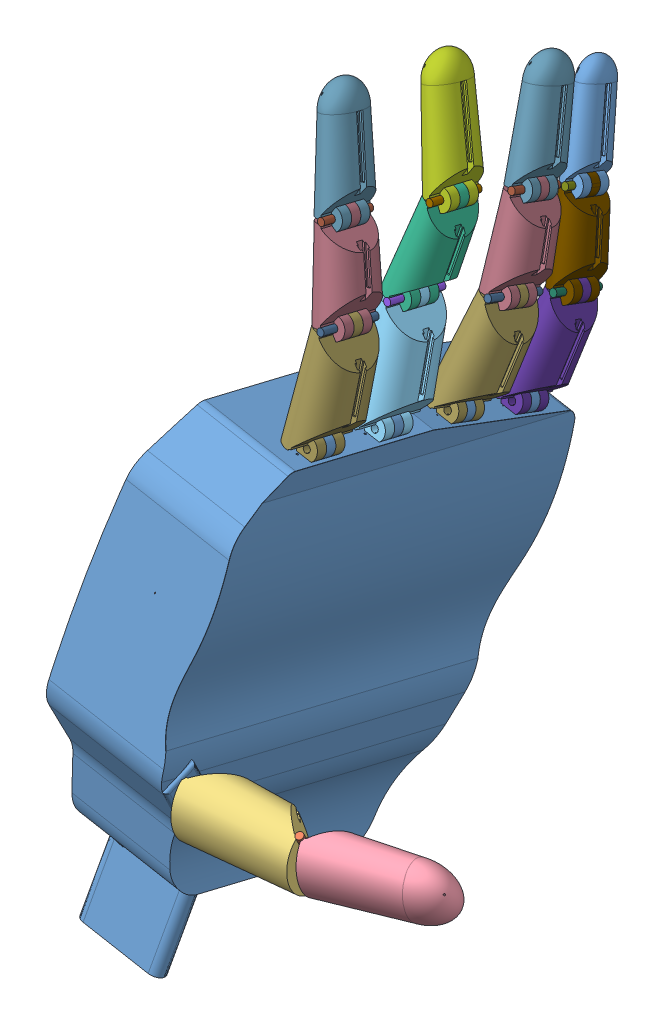
SolidWorks assembly hand_ass_son, configuration Default. Lengths in mm.
Overall size (126.68 238.36 164.71).
29 component instances, 20 part files, 48 mates.
Components (placement in the parent):
- mainbody_v2-4: mainbody_v2 [Default] at (1393.0939 256.2845 230.0733) x (-0.03967 -0.262646 -0.964076) z (0.98509 -0.171926 0.006304) size (116.82 140 48.77)
- Mate1t-4: Mate1t [Default] at (1443.7902 225.3063 267.9284) x (0.146425 0.857082 0.493933) z (0.670742 0.280983 -0.686407) size (23 2 2)
- Part1t-3: Part1t [Default] at (1431.2867 235.9478 276.4521) x (0.146425 0.857082 0.493933) z (-0.086451 0.508491 -0.856716) size (25.41 37 18.49)
- Part2t-3: Part2t [Default] at (1462.1105 235.1801 268.6506) x (0.146425 0.857082 0.493933) z (-0.264208 0.51506 -0.815419) size (22.13 38.57 15.06)
- Part1m-2: Part1m [Default] at (1414.4402 322.5973 216.192) x (-0.03967 -0.262646 -0.964076) z (0.999177 -0.002227 -0.040508) size (21.28 37 15.36)
- Part2m-2: Part2m [Default] at (1416.9612 349.6562 208.7166) x (-0.03967 -0.262646 -0.964076) z (0.980971 -0.193758 0.012421) size (18.99 32 13.25)
- Part3m-2: Part3m [Default] at (1414.6092 375.7736 201.6979) x (-0.03967 -0.262646 -0.964076) z (0.948609 0.293255 -0.118926) size (16.1 35.5 11.04)
- Mate1-2: Mate1 [Default] at (1415.2589 339.0559 221.0098) x (-0.03967 -0.262646 -0.964076) z (0.870094 0.465305 -0.162567) size (18 2 2)
- Mate2-2: Mate2 [Default] at (1420.1608 363.3694 213.1471) x (-0.03967 -0.262646 -0.964076) z (0.88018 0.447523 -0.158138) size (16 2 2)
- Mate1i-7: Mate1i [Default] at (1419.1567 328.7029 194.6213) x (-0.061096 -0.383846 -0.921374) z (0.853883 0.457912 -0.247388) size (18 2 2)
- Mate2i-7: Mate2i [Default] at (1415.3779 344.2512 169.9444) x (0.061096 0.383846 0.921374) z (-0.994886 0.097798 0.025228) size (16 2 2)
- Part1i-6: Part1i [Default] at (1415.7923 312.9467 191.6404) x (-0.061096 -0.383846 -0.921374) z (0.98509 -0.171926 0.006304) size (21.16 35 15.37)
- Part2-6: Part2 [Default] at (1416.6054 336.7334 181.6776) x (-0.061096 -0.383846 -0.921374) z (0.991581 0.082247 -0.100016) size (18.98 30 13.22)
- Part3i-6: Part3i [Default] at (1412.8163 360.7728 171.9137) x (-0.061096 -0.383846 -0.921374) z (0.980311 0.150581 -0.127736) size (16.1 33.51 11.04)
- Mate1p-2: Mate1p [Default] at (1417.5601 318.7755 173.3582) x (-0.061096 -0.383846 -0.921374) z (0.991721 -0.127797 -0.01252) size (16 2 2)
- Mate2p-2: Mate2p [Default] at (1411.96 339.126 164.166) x (-0.061096 -0.383846 -0.921374) z (0.997555 0.007899 -0.069439) size (14 2 2)
- Part1p-2: Part1p [Default] at (1414.4302 303.698 171.1644) x (-0.061096 -0.383846 -0.921374) z (0.98509 -0.171926 0.006304) size (18.99 34 13.27)
- Part2p-2: Part2p [Default] at (1413.7865 326.3018 161.7901) x (-0.061096 -0.383846 -0.921374) z (0.968644 0.199919 -0.147517) size (16.86 29 11.21)
- Part3p-2: Part3p [Default] at (1408.3506 348.6966 152.8208) x (-0.061096 -0.383846 -0.921374) z (0.974142 0.178236 -0.138849) size (14.11 31.5 9.04)
- Mate1i-8: Mate1i [Default] at (1416.3045 338.1976 225.4891) x (0.03967 0.262646 0.964076) z (-0.987081 -0.139593 0.078646) size (18 2 2)
- Mate2i-8: Mate2i [Default] at (1409.7839 360.8016 220.6372) x (0.03967 0.262646 0.964076) z (-0.919513 -0.368003 0.138092) size (16 2 2)
- Part1i-7: Part1i [Default] at (1415.7465 327.3903 237.7916) x (-0.03967 -0.262646 -0.964076) z (0.998985 -0.031014 -0.032657) size (21.16 35 15.37)
- Part3i-7: Part3i [Default] at (1405.8994 376.6502 224.7772) x (-0.03967 -0.262646 -0.964076) z (0.963202 0.246636 -0.106826) size (16.1 33.51 11.04)
- Part2-7: Part2 [Default] at (1412.6818 352.0877 231.19) x (-0.03967 -0.262646 -0.964076) z (0.961097 0.253914 -0.108722) size (18.98 30 13.22)
- SERVO 2-2: SERVO 2 [Default] at (1378.4658 252.7443 237.0888) x (0.374746 0.816954 0.438351) z (0.900147 -0.433837 0.039007) size (32 28.96 12.1)
- SERVO 2-3: SERVO 2 [Default] at (1410.6392 255.7893 252.4191) x (0.348093 0.174989 0.920983) z (-0.929377 0.193147 0.314567) size (32 28.96 12.1)
- SERVO 2-4: SERVO 2 [Default] at (1411.5824 241.8867 212.5876) x (0.093781 0.315033 0.944436) z (-0.990432 0.125987 0.056324) size (32 28.96 12.1)
- SERVO 2-6: SERVO 2 [Default] at (1414.0198 249.6937 180.1774) x (0.274408 0.279911 0.919973) z (-0.954781 0.193152 0.226022) size (32 28.96 12.1)
- SERVO 2-7: SERVO 2 [Default] at (1409.5967 265.7988 229.5325) x (0.0903 0.334214 0.938161) z (-0.97905 0.202412 0.022128) size (32 28.96 12.1)
Mates (geometry in assembly coordinates):
- Concentric1: concentric anti-aligned: cylinder of mainbody_v2-4 through (1415.9837 312.2001 240.3647) axis (0.03967 0.262646 0.964076) radius 1; cylinder of Part1i-7 through (1416.4652 315.3881 252.0667) axis (-0.03967 -0.262646 -0.964076) radius 1
- Coincident1: coincident anti-aligned: plane of mainbody_v2-4 through (1415.9837 312.2001 240.3647) normal (-0.03967 -0.262646 -0.964076); plane of Part1i-7 through (1415.9837 312.2001 240.3647) normal (0.03967 0.262646 0.964076)
- Concentric4: concentric aligned: cylinder of Part1i-7 through (1417.0836 343.3556 244.4221) axis (-0.03967 -0.262646 -0.964076) radius 1; cylinder of Part2-7 through (1417.0387 343.0583 243.331) axis (-0.03967 -0.262646 -0.964076) radius 1
- Coincident4: coincident anti-aligned: plane of Part1i-7 through (1416.6021 340.1676 232.72) normal (-0.03967 -0.262646 -0.964076); plane of Part2-7 through (1416.6021 340.1676 232.72) normal (0.03967 0.262646 0.964076)
- Concentric5: concentric aligned: cylinder of Mate1i-8 through (1417.0186 342.9252 242.8424) axis (-0.03967 -0.262646 -0.964076) radius 1; cylinder of Part2-7 through (1417.0387 343.0583 243.331) axis (-0.03967 -0.262646 -0.964076) radius 1
- Coincident5: coincident anti-aligned: plane of Mate1i-8 through (1416.6616 340.5614 234.1658) normal (0.03967 0.262646 0.964076); plane of Part1i-7 through (1415.7465 327.3903 237.7916) normal (-0.03967 -0.262646 -0.964076)
- Concentric6: concentric anti-aligned: cylinder of Part3i-7 through (1409.8037 360.9329 221.1191) axis (0.03967 0.262646 0.964076) radius 1; cylinder of Part2-7 through (1410.4784 365.3995 237.5145) axis (-0.03967 -0.262646 -0.964076) radius 1
- Coincident6: coincident anti-aligned: plane of Part3i-7 through (1410.0417 362.5088 226.9035) normal (0.03967 0.262646 0.964076); plane of Part2-7 through (1410.0417 362.5088 226.9035) normal (-0.03967 -0.262646 -0.964076)
- Concentric8: concentric anti-aligned: cylinder of Mate2i-8 through (1410.4186 365.004 236.0624) axis (-0.03967 -0.262646 -0.964076) radius 1; cylinder of Part3i-7 through (1409.8037 360.9329 221.1191) axis (0.03967 0.262646 0.964076) radius 1
- Coincident8: coincident anti-aligned: plane of Mate2i-8 through (1410.1012 362.9028 228.3498) normal (0.03967 0.262646 0.964076); plane of Part2-7 through (1412.6818 352.0877 231.19) normal (-0.03967 -0.262646 -0.964076)
- Concentric9: concentric anti-aligned: cylinder of mainbody_v2-4 through (1415.1056 306.3865 219.0249) axis (0.03967 0.262646 0.964076) radius 1; cylinder of Part1m-2 through (1415.5873 309.5752 230.7296) axis (-0.03967 -0.262646 -0.964076) radius 1
- Coincident9: coincident anti-aligned: plane of mainbody_v2-4 through (1415.1056 306.3865 219.0249) normal (-0.03967 -0.262646 -0.964076); plane of Part1m-2 through (1415.1056 306.3865 219.0249) normal (0.03967 0.262646 0.964076)
- Concentric10: concentric aligned: cylinder of Part1m-2 through (1415.324 339.4868 222.5916) axis (-0.03967 -0.262646 -0.964076) radius 1; cylinder of Part2m-2 through (1415.2792 339.1899 221.5017) axis (-0.03967 -0.262646 -0.964076) radius 1
- Coincident10: coincident anti-aligned: plane of Part1m-2 through (1414.8424 336.2981 210.8869) normal (-0.03967 -0.262646 -0.964076); plane of Part2m-2 through (1414.8424 336.2981 210.8869) normal (0.03967 0.262646 0.964076)
- Concentric11: concentric anti-aligned: cylinder of Part2m-2 through (1415.2792 339.1899 221.5017) axis (-0.03967 -0.262646 -0.964076) radius 1; cylinder of Mate1-2 through (1414.5449 334.3282 203.6564) axis (0.03967 0.262646 0.964076) radius 1
- Coincident12: coincident aligned: plane of Part1m-2 through (1414.4402 322.5973 216.192) normal (-0.03967 -0.262646 -0.964076); plane of Mate1-2 through (1414.9019 336.6921 212.3331) normal (-0.03967 -0.262646 -0.964076)
- Concentric12: concentric anti-aligned: cylinder of Part2m-2 through (1420.2207 363.7661 214.603) axis (-0.03967 -0.262646 -0.964076) radius 1; cylinder of Part3m-2 through (1419.5459 359.2984 198.2037) axis (0.03967 0.262646 0.964076) radius 1
- Coincident13: coincident anti-aligned: plane of Part2m-2 through (1419.7839 360.8743 203.9882) normal (-0.03967 -0.262646 -0.964076); plane of Part3m-2 through (1419.7839 360.8743 203.9882) normal (0.03967 0.262646 0.964076)
- Concentric13: concentric aligned: cylinder of Part3m-2 through (1419.5459 359.2984 198.2037) axis (0.03967 0.262646 0.964076) radius 1; cylinder of Mate2-2 through (1419.5261 359.1671 197.7219) axis (0.03967 0.262646 0.964076) radius 1
- Coincident14: coincident aligned: plane of Part2m-2 through (1416.9612 349.6562 208.7166) normal (-0.03967 -0.262646 -0.964076); plane of Mate2-2 through (1419.8435 361.2683 205.4345) normal (-0.03967 -0.262646 -0.964076)
- Parallel2: parallel anti-aligned: plane of mainbody_v2-4 through (1383.8165 307.0595 209.2378) normal (0.160828 0.907251 -0.388627); plane of Part1i-6 through (1414.6286 303.2312 206.6189) normal (-0.160828 -0.907251 0.388627)
- Concentric14: concentric aligned: cylinder of mainbody_v2-4 through (1414.0344 299.5139 198.9816) axis (-0.061096 -0.383846 -0.921374) radius 1; cylinder of Part1i-6 through (1414.5927 303.0215 207.4011) axis (-0.061096 -0.383846 -0.921374) radius 1
- Coincident17: coincident anti-aligned: plane of mainbody_v2-4 through (1413.8511 298.3624 196.2174) normal (-0.061096 -0.383846 -0.921374); plane of Part1i-6 through (1413.8511 298.3624 196.2174) normal (0.061096 0.383846 0.921374)
- Concentric15: concentric aligned: cylinder of Part1i-6 through (1419.2568 329.3318 196.131) axis (-0.061096 -0.383846 -0.921374) radius 1; cylinder of Part2-6 through (1419.1876 328.8974 195.0882) axis (-0.061096 -0.383846 -0.921374) radius 1
- Coincident18: coincident anti-aligned: plane of Part1i-6 through (1418.6985 325.8242 187.7114) normal (0.061096 0.383846 0.921374); plane of Part2-6 through (1418.6985 325.8242 187.7114) normal (-0.061096 -0.383846 -0.921374)
- Concentric16: concentric anti-aligned: cylinder of Mate1i-7 through (1418.0569 321.7936 178.0366) axis (0.061096 0.383846 0.921374) radius 1; cylinder of Part2-6 through (1419.1876 328.8974 195.0882) axis (-0.061096 -0.383846 -0.921374) radius 1
- Coincident20: coincident aligned: plane of Mate1i-7 through (1418.6068 325.2483 186.329) normal (-0.061096 -0.383846 -0.921374); plane of Part1i-6 through (1415.7923 312.9467 191.6404) normal (-0.061096 -0.383846 -0.921374)
- Concentric17: concentric anti-aligned: cylinder of Part2-6 through (1416.4475 350.9708 186.0741) axis (-0.061096 -0.383846 -0.921374) radius 1; cylinder of Part3i-6 through (1415.4085 344.443 170.4049) axis (0.061096 0.383846 0.921374) radius 1
- Coincident21: coincident anti-aligned: plane of Part2-6 through (1415.9583 347.8976 178.6973) normal (0.061096 0.383846 0.921374); plane of Part3i-6 through (1415.9583 347.8976 178.6973) normal (-0.061096 -0.383846 -0.921374)
- Concentric18: concentric anti-aligned: cylinder of Mate2i-7 through (1416.3555 350.3927 184.6864) axis (-0.061096 -0.383846 -0.921374) radius 1; cylinder of Part3i-6 through (1415.4085 344.443 170.4049) axis (0.061096 0.383846 0.921374) radius 1
- Coincident22: coincident anti-aligned: plane of Mate2i-7 through (1415.8667 347.3219 177.3154) normal (0.061096 0.383846 0.921374); plane of Part2-6 through (1416.6054 336.7334 181.6776) normal (-0.061096 -0.383846 -0.921374)
- Parallel3: parallel anti-aligned: plane of mainbody_v2-4 through (1383.8165 307.0595 209.2378) normal (0.160828 0.907251 -0.388627); plane of Part1p-2 through (1413.1864 294.2119 184.9666) normal (-0.160828 -0.907251 0.388627)
- Concentric19: concentric aligned: cylinder of mainbody_v2-4 through (1412.6598 290.8774 178.2507) axis (-0.061096 -0.383846 -0.921374) radius 1; cylinder of Part1p-2 through (1413.1494 293.9534 185.6343) axis (-0.061096 -0.383846 -0.921374) radius 1
- Coincident24: coincident anti-aligned: plane of mainbody_v2-4 through (1412.4765 289.7259 175.4865) normal (-0.061096 -0.383846 -0.921374); plane of Part1p-2 through (1412.4765 289.7259 175.4865) normal (0.061096 0.383846 0.921374)
- Concentric20: concentric aligned: cylinder of Part1p-2 through (1417.6526 319.3565 174.7528) axis (-0.061096 -0.383846 -0.921374) radius 1; cylinder of Part2p-2 through (1417.5885 318.954 173.7868) axis (-0.061096 -0.383846 -0.921374) radius 1
- Coincident25: coincident anti-aligned: plane of Part1p-2 through (1416.9797 315.1289 164.605) normal (-0.061096 -0.383846 -0.921374); plane of Part2p-2 through (1416.9797 315.1289 164.605) normal (0.061096 0.383846 0.921374)
- Concentric21: concentric anti-aligned: cylinder of Mate1p-2 through (1416.5826 312.6339 158.6162) axis (0.061096 0.383846 0.921374) radius 1; cylinder of Part2p-2 through (1417.5885 318.954 173.7868) axis (-0.061096 -0.383846 -0.921374) radius 1
- Coincident26: coincident aligned: plane of Mate1p-2 through (1417.0713 315.7047 165.9872) normal (-0.061096 -0.383846 -0.921374); plane of Part1p-2 through (1414.4302 303.698 171.1644) normal (-0.061096 -0.383846 -0.921374)
- Concentric22: concentric anti-aligned: cylinder of Part2p-2 through (1412.0496 339.6884 165.5161) axis (-0.061096 -0.383846 -0.921374) radius 1; cylinder of Part3p-2 through (1411.0742 333.5602 150.806) axis (0.061096 0.383846 0.921374) radius 1
- Coincident27: coincident anti-aligned: plane of Part2p-2 through (1411.4407 335.8633 156.3343) normal (-0.061096 -0.383846 -0.921374); plane of Part3p-2 through (1411.4407 335.8633 156.3343) normal (0.061096 0.383846 0.921374)
- Concentric24: concentric aligned: cylinder of Mate2p-2 through (1411.1047 333.7521 151.2667) axis (0.061096 0.383846 0.921374) radius 1; cylinder of Part3p-2 through (1411.0742 333.5602 150.806) axis (0.061096 0.383846 0.921374) radius 1
- Coincident28: coincident aligned: plane of Mate2p-2 through (1411.5324 336.439 157.7163) normal (-0.061096 -0.383846 -0.921374); plane of Part2p-2 through (1413.7865 326.3018 161.7901) normal (-0.061096 -0.383846 -0.921374)
- Concentric25: concentric anti-aligned: cylinder of mainbody_v2-4 through (1415.1452 239.0135 278.9547) axis (-0.146425 -0.857082 -0.493933) radius 1; cylinder of Part1t-3 through (1413.0554 226.7806 271.9049) axis (0.146425 0.857082 0.493933) radius 1
- Concentric27: concentric anti-aligned: cylinder of Part1t-3 through (1443.6039 224.2155 267.2998) axis (0.146425 0.857082 0.493933) radius 1; cylinder of Part2t-3 through (1446.5723 241.591 277.3132) axis (-0.146425 -0.857082 -0.493933) radius 1
- Coincident30: coincident anti-aligned: plane of mainbody_v2-4 through (1415.1452 239.0135 278.9547) normal (0.146425 0.857082 0.493933); plane of Part1t-3 through (1415.1452 239.0135 278.9547) normal (-0.146425 -0.857082 -0.493933)
- Coincident32: coincident anti-aligned: plane of Part1t-3 through (1445.6938 236.4485 274.3496) normal (0.146425 0.857082 0.493933); plane of Part2t-3 through (1445.6938 236.4485 274.3496) normal (-0.146425 -0.857082 -0.493933)
- Concentric28: concentric aligned: cylinder of Mate1t-4 through (1447.158 245.0192 279.2888) axis (-0.146425 -0.857082 -0.493933) radius 1; cylinder of Part2t-3 through (1446.5723 241.591 277.3132) axis (-0.146425 -0.857082 -0.493933) radius 1
- Coincident33: coincident aligned: plane of Mate1t-4 through (1445.4741 235.1627 273.6086) normal (0.146425 0.857082 0.493933); plane of Part1t-3 through (1431.2867 235.9478 276.4521) normal (0.146425 0.857082 0.493933)
